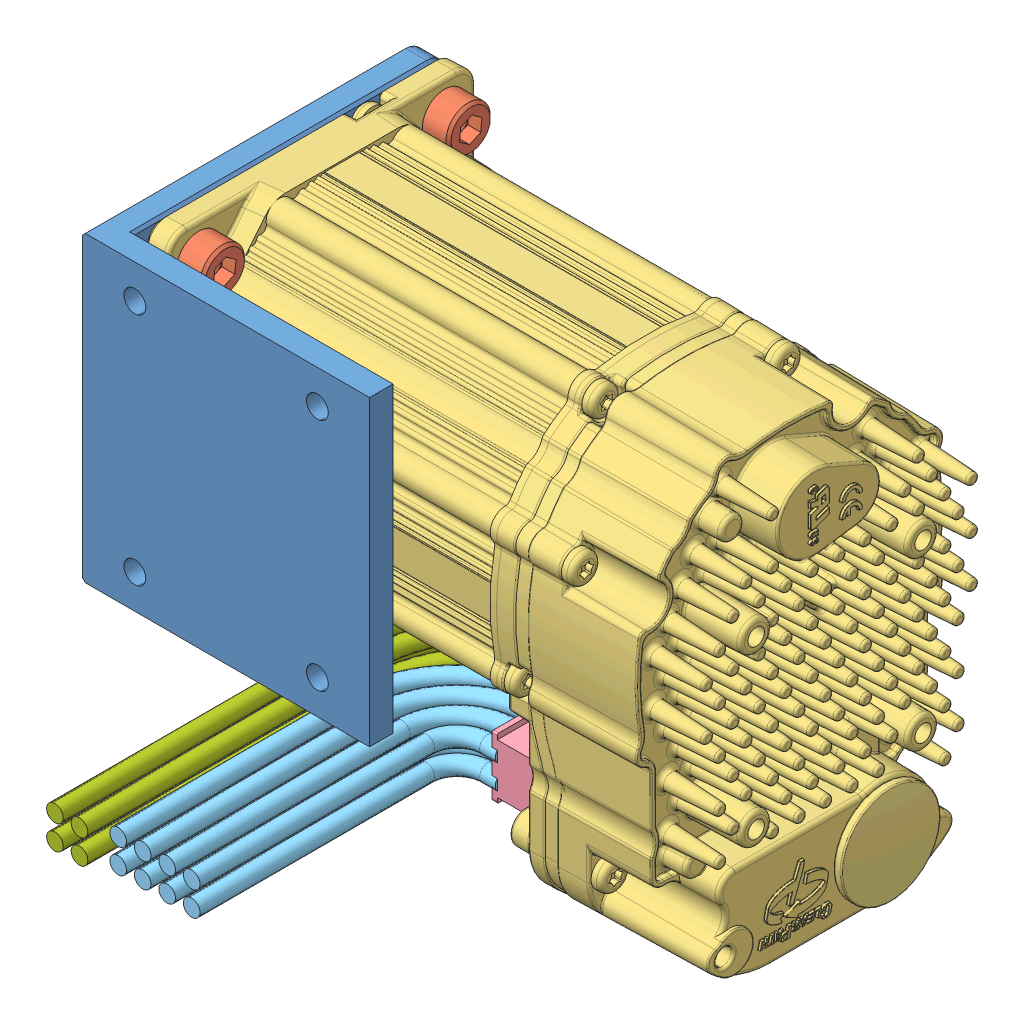
SolidWorks assembly motor_assembly, configuration Default. Lengths in mm.
Overall size (124.71 82.13 99.26).
12 component instances, 7 part files, 20 mates.
Components (placement in the parent):
- motor_angle_bracket-1: motor_angle_bracket [Default] at origin size (55 58 65)
- socket head cap screw_am-1: socket head cap screw_am [B18.3.1M - 5 x 0.8 x 10 Hex SHCS -- 10NHX] at (14.819 52.5732 -59.5732) x (-1 0 0) z (0 -0.909932 -0.414757) size (15 8.5 8.5)
- socket head cap screw_am-2: socket head cap screw_am [B18.3.1M - 5 x 0.8 x 10 Hex SHCS -- 10NHX] at (14.819 5.4268 -59.5732) x (-1 0 0) z (0 -0.909932 -0.414757) size (15 8.5 8.5)
- socket head cap screw_am-3: socket head cap screw_am [B18.3.1M - 5 x 0.8 x 10 Hex SHCS -- 10NHX] at (14.819 5.4268 -12.4268) x (-1 0 0) z (0 -0.909932 -0.414757) size (15 8.5 8.5)
- socket head cap screw_am-4: socket head cap screw_am [B18.3.1M - 5 x 0.8 x 10 Hex SHCS -- 10NHX] at (14.819 52.5732 -12.4268) x (-1 0 0) z (0 -0.909932 -0.414757) size (15 8.5 8.5)
- CPM-_ _ _ _ -2321_-LS-1: CPM-_ _ _ _ -2321_-LS [Default] at (80.334 29 -36) x (0 1 0) z (1 0 0) size (82.13 59.99 124.71)
- clearpath_data_loom-1: clearpath_data_loom [Default] at (61.0589 2.274 -42.6649) x (0 0 1) z (1 0 0) size (67.7 14.4 59.2)
  - 39-01-3085-1: 39-01-3085 [Default] at (15.1122 12.208 9.586) size (18 14.4 19.6)
  - microfit_4x2_loom-1: microfit_4x2_loom [Default] at (8.8122 10.183 -0.114) x (0 0 -1) z (1 0 0) size (40.6 7.9 66.6)
- clearpath_power_loom-1: clearpath_power_loom [Default] at (70.645 -9.934 -48.6359) x (0 0 1) z (1 0 0) size (86.7 14.4 68.2)
  - 39-01-3045-1: 39-01-3045 [Default] at origin size (9.6 14.4 19.6)
  - microfit_2x2_loom-1: microfit_2x2_loom [Default] at (-2.1 -2.025 -9.7) x (0 0 -1) z (1 0 0) size (49.6 7.9 85.6)
Mates (geometry in assembly coordinates):
- Concentric24: concentric anti-aligned: cylinder of motor_angle_bracket-1 through (0 52.5732 -59.5732) axis (-1 0 0) radius 2.1; cylinder of socket head cap screw_am-1 through (46.569 52.5732 -59.5732) axis (1 0 0) radius 2.5
- Coincident484: coincident anti-aligned: plane of motor_angle_bracket-1 through (5 58 -65) normal (1 0 0); plane of CPM-_ _ _ _ -2321_-LS-1 through (5 29 -36) normal (-1 0 0)
- Concentric182: concentric anti-aligned: cylinder of socket head cap screw_am-2 through (46.569 5.4268 -59.5732) axis (1 0 0) radius 2.5; cylinder of CPM-_ _ _ _ -2321_-LS-1 through (17.5 5.4268 -59.5732) axis (-1 0 0) radius 2.6
- Concentric183: concentric anti-aligned: cylinder of socket head cap screw_am-1 through (46.569 52.5732 -59.5732) axis (1 0 0) radius 2.5; cylinder of CPM-_ _ _ _ -2321_-LS-1 through (17.5 52.5732 -59.5732) axis (-1 0 0) radius 2.6
- Concentric184: concentric anti-aligned: cylinder of socket head cap screw_am-3 through (46.569 5.4268 -12.4268) axis (1 0 0) radius 2.5; cylinder of CPM-_ _ _ _ -2321_-LS-1 through (17.5 5.4268 -12.4268) axis (-1 0 0) radius 2.6
- Concentric185: concentric anti-aligned: cylinder of socket head cap screw_am-4 through (46.569 52.5732 -12.4268) axis (1 0 0) radius 2.5; cylinder of CPM-_ _ _ _ -2321_-LS-1 through (17.5 52.5732 -12.4268) axis (-1 0 0) radius 2.6
- Coincident486: coincident anti-aligned: plane of socket head cap screw_am-4 through (9.819 54.3359 -16.294) normal (-1 0 0); plane of CPM-_ _ _ _ -2321_-LS-1 through (9.819 44.0593 -16.1691) normal (1 0 0)
- Coincident487: coincident anti-aligned: plane of socket head cap screw_am-1 through (9.819 54.3359 -63.4404) normal (-1 0 0); plane of CPM-_ _ _ _ -2321_-LS-1 through (9.819 48.8309 -51.0593) normal (1 0 0)
- Coincident488: coincident anti-aligned: plane of socket head cap screw_am-2 through (9.819 7.1895 -63.4404) normal (-1 0 0); plane of CPM-_ _ _ _ -2321_-LS-1 through (9.819 13.9407 -55.8309) normal (1 0 0)
- Coincident489: coincident anti-aligned: plane of socket head cap screw_am-3 through (9.819 7.1895 -16.294) normal (-1 0 0); plane of CPM-_ _ _ _ -2321_-LS-1 through (9.819 9.1691 -20.9407) normal (1 0 0)
- Concentric186: concentric anti-aligned: cylinder of motor_angle_bracket-1 through (0 29 -36) axis (1 0 0) radius 20; cylinder of CPM-_ _ _ _ -2321_-LS-1 through (5 29 -36) axis (-1 0 0) radius 19.05
- Width1: width anti-aligned: plane of CPM-_ _ _ _ -2321_-LS-1 through (70.645 -5.984 -19.5027) normal (0 1 0); plane of CPM-_ _ _ _ -2321_-LS-1 through (70.645 -13.684 -23.0027) normal (0 -1 0); plane of clearpath_data_loom-1/39-01-3085-1 through (70.645 -13.634 -19.5527) normal (0 -1 0); plane of clearpath_data_loom-1/39-01-3085-1 through (70.645 -6.034 -22.9527) normal (0 1 0)
- Width2: width anti-aligned: plane of CPM-_ _ _ _ -2321_-LS-1 through (79.745 -13.684 -48.2859) normal (0 1 0); plane of CPM-_ _ _ _ -2321_-LS-1 through (79.745 -5.984 -44.7859) normal (0 -1 0); plane of clearpath_power_loom-1/39-01-3045-1 through (70.645 -13.634 -44.8359) normal (0 -1 0); plane of clearpath_power_loom-1/39-01-3045-1 through (70.645 -6.034 -47.4859) normal (0 1 0)
- Width3: width anti-aligned: plane of CPM-_ _ _ _ -2321_-LS-1 through (79.745 -9.484 -44.7859) normal (0 0 -1); plane of CPM-_ _ _ _ -2321_-LS-1 through (79.745 -5.984 -52.4859) normal (0 0 1); plane of clearpath_power_loom-1/39-01-3045-1 through (70.645 -6.784 -44.8359) normal (0 0 1); plane of clearpath_power_loom-1/39-01-3045-1 through (70.645 -9.434 -52.4359) normal (0 0 -1)
- Width4: width aligned: plane of clearpath_data_loom-1/39-01-3085-1 through (70.645 -9.434 -35.5527) normal (0 0 -1); plane of clearpath_data_loom-1/39-01-3085-1 through (70.645 -6.034 -19.5527) normal (0 0 1); plane of CPM-_ _ _ _ -2321_-LS-1 through (70.645 -5.984 -35.6027) normal (0 0 -1); plane of CPM-_ _ _ _ -2321_-LS-1 through (70.645 -9.484 -19.5027) normal (0 0 1)
- Coincident490: coincident aligned: plane of CPM-_ _ _ _ -2321_-LS-1 through (70.645 -14.434 -18.5527) normal (1 0 0); plane of clearpath_data_loom-1/39-01-3085-1 through (70.645 -14.734 -36.5527) normal (1 0 0)
- Coincident491: coincident anti-aligned: plane of CPM-_ _ _ _ -2321_-LS-1 through (70.645 -7.034 -53.4359) normal (-1 0 0); plane of clearpath_power_loom-1/39-01-3045-1 through (70.645 -14.734 -53.4359) normal (1 0 0)
- Coincident492: coincident aligned: plane of motor_angle_bracket-1 through (55 58 0) normal (0 0 1); plane of assembly through (0 0 0) normal (0 0 1)
- Coincident493: coincident anti-aligned: plane of motor_angle_bracket-1 through (0 0 0) normal (0 -1 0); plane of assembly through (0 0 0) normal (0 1 0)
- Coincident494: coincident anti-aligned: plane of motor_angle_bracket-1 through (0 58 0) normal (-1 0 0); plane of assembly through (0 0 0) normal (1 0 0)
